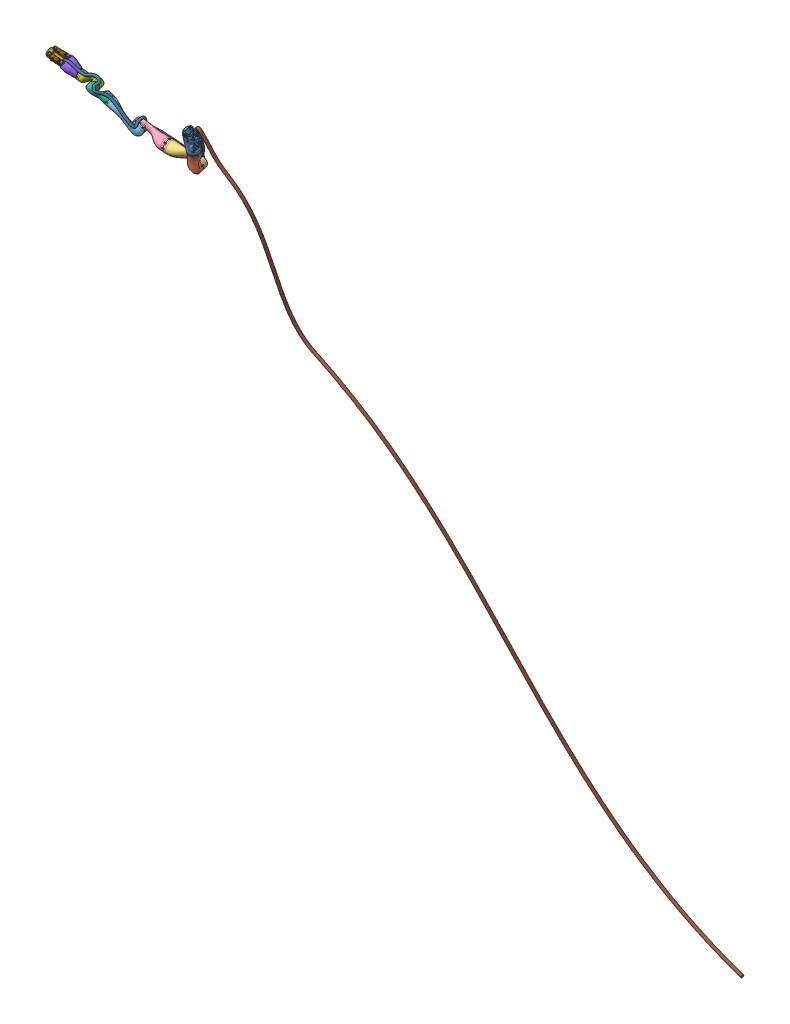
SolidWorks assembly AssemblyWMates_bckp, configuration Default. Lengths in mm.
Overall size (4116.45 4988.8 1804.64).
14 component instances, 12 part files, 30 mates.
Components (placement in the parent):
- Link_1-1: Link_1 [Default] at (138.4866 417.4377 297.5521) x (0.03698 0.287291 -0.957129) z (-0.087201 -0.953203 -0.289482) size (86.63 89.66 156.6)
- Link_2-1: Link_2 [Default] at (138.5302 417.9143 297.6968) x (0.023153 -0.292449 0.956001) z (-0.087201 -0.953203 -0.289482) size (82.77 82.53 159.85)
- Link_3-1: Link_3 [Default] at (387.9844 125.6422 202.7698) x (0.023153 -0.292449 0.956001) z (-0.992619 0.107145 0.056816) size (85.03 82.68 246.21)
- Link_4-1: Link_4 [Default] at (388.4749 125.5421 202.7265) x (0.019798 -0.319039 0.947535) z (-0.992619 0.107145 0.056816) size (85.03 82.68 246.21)
- Link_5-1: Link_5 [Default] at (239.1018 -208.1509 92.9641) x (0.019798 -0.319039 0.947535) z (-0.774729 0.594165 0.216245) size (63.11 82.51 248.26)
- Link_6-1: Link_6 [Default] at (239.5892 -214.9998 111.2165) x (0.009536 0.352942 -0.935597) z (-0.774729 0.594165 0.216245) size (79.26 63.11 135.28)
- Link_7-1: Link_7 [Default] at (435.3893 151.7526 252.0992) x (0.009536 0.352942 -0.935597) z (-0.971222 0.225948 0.075337) size (79.26 63.11 135.28)
- Palm-1: Palm [Default] at (433.6485 146.2609 239.4909) x (0.237886 0.904603 0.353699) z (-0.971222 0.225948 0.075337) size (117.9 99.6 122.71)
- Finger-1: Finger [Default] at (-29.239 -467.0767 -123.4465) x (0.80391 0.582407 0.120544) z (-0.580797 0.725108 0.369991) size (73.19 31.73 75.64)
- Finger-2: Finger [Default] at (319.2901 1059.8577 281.9942) x (0.507306 -0.86175 -0.005255) z (-0.861107 -0.507147 0.036001) size (73.19 31.73 75.64)
- Finger-3: Finger [Default] at (343.0635 944.2648 607.3154) x (0.468613 -0.837857 -0.279995) z (-0.881956 -0.425583 -0.202567) size (73.19 31.73 75.64)
- Part4^AssemblyWMates_bckp-1: Part4^AssemblyWMates_bckp [Default] at (138.4866 417.4377 297.5521) x (-0.03698 -0.287291 0.957129) z (0.087201 0.953203 0.289482) size (166.68 918.69 328.06) (virtual)
- Part5^AssemblyWMates_bckp-1: Part5^AssemblyWMates_bckp [Default] at (134.4689 373.5198 284.2145) x (-0.03698 -0.287291 0.957129) z (0.087201 0.953203 0.289482) size (401.21 3230.32 4793.68) (virtual)
- aruco_marker_holderHose-1: aruco_marker_holderHose [Default] at (-711.4651 422.1788 332.2532) x (0.237886 0.904603 0.353699) z (-0.011767 -0.361442 0.93232) size (60 115.16 60)
Mates (geometry in assembly coordinates):
- Concentric1: concentric anti-aligned: cylinder of Link_2-1 through (124.8397 268.2614 252.2482) axis (0.087201 0.953203 0.289482) radius 37.25; cylinder of Link_1-1 through (124.8397 268.2614 252.2482) axis (-0.087201 -0.953203 -0.289482) radius 37.25
- Coincident2: coincident anti-aligned: plane of Link_2-1 through (86.5196 275.7995 238.97) normal (0.087201 0.953203 0.289482); plane of Link_1-1 through (139.1451 255.8263 288.8854) normal (-0.087201 -0.953203 -0.289482)
- Concentric5: concentric anti-aligned: cylinder of Link_2-1 through (114.4717 155.7455 216.5106) axis (-0.023153 0.292449 -0.956001) radius 37.25; cylinder of Link_3-1 through (114.4717 155.7455 216.5106) axis (0.023153 -0.292449 0.956001) radius 37.25
- Coincident4: coincident anti-aligned: plane of Link_2-1 through (75.1406 143.6201 213.7539) normal (-0.023153 0.292449 -0.956001); plane of Link_3-1 through (134.6777 190.2686 226.5822) normal (0.023153 -0.292449 0.956001)
- Concentric7: concentric anti-aligned: cylinder of Link_3-1 through (-88.7612 177.6103 228.3828) axis (-0.992619 0.107145 0.056816) radius 37.25; cylinder of Link_4-1 through (-88.7612 177.6103 228.3828) axis (0.992619 -0.107145 -0.056816) radius 37.25
- Coincident7: coincident anti-aligned: plane of Link_3-1 through (-83.8589 209.2082 254.4423) normal (-0.992619 0.107145 0.056816); plane of Link_4-1 through (-93.0086 136.6872 231.3523) normal (0.992619 -0.107145 -0.056816)
- Concentric9: concentric anti-aligned: cylinder of Link_4-1 through (-292.0048 199.628 239.779) axis (0.019798 -0.319039 0.947535) radius 37.25; cylinder of Link_5-1 through (-292.0048 199.628 239.779) axis (-0.019798 0.319039 -0.947535) radius 37.25
- Coincident6: coincident anti-aligned: plane of Link_4-1 through (-312.2339 165.4325 228.6879) normal (0.019798 -0.319039 0.947535); plane of Link_5-1 through (-303.8601 162.1096 227.3941) normal (-0.019798 0.319039 -0.947535)
- Concentric11: concentric anti-aligned: cylinder of Link_5-1 through (-452.1511 319.031 295.2016) axis (-0.774729 0.594165 0.216245) radius 29; cylinder of Link_6-1 through (-452.1511 319.031 295.2016) axis (0.774729 -0.594165 -0.216245) radius 29
- Coincident8: coincident anti-aligned: plane of Link_5-1 through (-432.2436 342.2895 302.6169) normal (-0.774729 0.594165 0.216245); plane of Link_6-1 through (-472.066 296.2637 286.4099) normal (0.774729 -0.594165 -0.216245)
- Concentric18: concentric anti-aligned: cylinder of Link_6-1 through (-532.3379 380.4389 317.8169) axis (0.009536 0.352942 -0.935597) radius 29; cylinder of Link_7-1 through (-532.3379 380.4389 317.8169) axis (-0.009536 -0.352942 0.935597) radius 29
- Coincident9: coincident anti-aligned: plane of Link_6-1 through (-552.2529 357.6716 309.0252) normal (0.009536 0.352942 -0.935597); plane of Link_7-1 through (-539.8345 351.8384 306.9513) normal (-0.009536 -0.352942 0.935597)
- Concentric21: concentric anti-aligned: cylinder of Link_7-1 through (-632.8618 403.7363 325.8482) axis (-0.971222 0.225948 0.075337) radius 29; cylinder of Palm-1 through (-632.8618 403.7363 325.8482) axis (0.971222 -0.225948 -0.075337) radius 29
- Coincident10: coincident anti-aligned: plane of Link_7-1 through (-640.3583 375.1358 314.9826) normal (-0.971222 0.225948 0.075337); plane of Palm-1 through (-632.4911 415.1217 296.4801) normal (0.971222 -0.225948 -0.075337)
- Concentric23: concentric aligned: cylinder of Palm-1 through (-750.761 390.7291 342.046) axis (-0.044366 0.533346 -0.844733) radius 1.5; cylinder of Finger-1 through (-752.2779 408.965 313.1634) axis (-0.044366 0.533346 -0.844733) radius 2.5
- Coincident13: coincident anti-aligned: plane of Palm-1 through (-755.2752 408.4531 322.203) normal (-0.044366 0.533346 -0.844733); circle of Finger-1
- Concentric24: concentric aligned: cylinder of Palm-1 through (-738.5394 465.2212 304.6255) axis (0.034765 -0.186428 0.981853) radius 1.5; cylinder of Finger-2 through (-737.3508 458.847 338.1964) axis (0.034765 -0.186428 0.981853) radius 2.5
- Coincident14: coincident anti-aligned: plane of Palm-1 through (-742.6181 457.9619 330.2951) normal (0.034765 -0.186428 0.981853); circle of Finger-2
- Concentric25: concentric aligned: cylinder of Palm-1 through (-737.3339 455.5425 348.472) axis (-0.056567 -0.522567 0.85072) radius 1.5; cylinder of Finger-3 through (-739.268 437.6752 377.5592) axis (-0.056567 -0.522567 0.85072) radius 2.5
- Coincident15: coincident anti-aligned: plane of Palm-1 through (-742.9618 447.7103 356.7051) normal (0.056567 0.522567 -0.85072); circle of Finger-3
- InPlace1: in place: plane of Link_1-1 through (138.4866 417.4377 297.5521) normal (0.087201 0.953203 0.289482); plane of ? through (43.2615 472.8984 143.6161) normal (0.087201 0.953203 0.289482); moOrthogonalPlaneRef_w of Link_1-1 through (138.4866 417.4377 297.5521) normal (0.087201 0.953203 0.289482); plane of ? through (43.2615 472.8984 143.6161) normal (0 0.290588 -0.956848); plane of Link_1-1 through (138.4866 417.4377 297.5521) normal (0.087201 0.953203 0.289482); plane of ? through (43.2615 472.8984 143.6161) normal (0.996191 -0.083438 -0.025339); plane of Link_1-1 through (138.4866 417.4377 297.5521) normal (0.087201 0.953203 0.289482); unknown of Part4^AssemblyWMates_bckp-1
- Coincident17: coincident aligned: plane of Link_1-1; plane of Part4^AssemblyWMates_bckp-1
- Coincident18: coincident aligned: moOrthogonalPlaneRef_w of Link_1-1 through (138.4866 417.4377 297.5521) normal (0.995504 -0.094167 0.010198); plane of Part4^AssemblyWMates_bckp-1 through (138.4866 417.4377 297.5521) normal (0.995504 -0.094167 0.010198)
- Coincident19: coincident anti-aligned: moOrthogonalPlaneRef_w of Link_1-1 through (138.4866 417.4377 297.5521) normal (0.03698 0.287291 -0.957129); plane of Part4^AssemblyWMates_bckp-1 through (138.4866 417.4377 297.5521) normal (-0.03698 -0.287291 0.957129)
- InPlace2: in place: plane of Part4^AssemblyWMates_bckp-1 through (136.0236 385.366 244.739) normal (0.087201 0.953203 0.289482); plane of ? through (39.2438 428.9805 130.2786) normal (0.087201 0.953203 0.289482); plane of Part4^AssemblyWMates_bckp-1 through (136.0236 385.366 244.739) normal (0.087201 0.953203 0.289482); plane of ? through (39.2438 428.9805 130.2786) normal (0 0.290588 -0.956848); plane of Part4^AssemblyWMates_bckp-1 through (136.0236 385.366 244.739) normal (0.087201 0.953203 0.289482); plane of ? through (39.2438 428.9805 130.2786) normal (0.996191 -0.083438 -0.025339); plane of Part4^AssemblyWMates_bckp-1 through (136.0236 385.366 244.739) normal (0.087201 0.953203 0.289482); unknown of Part5^AssemblyWMates_bckp-1
- Coincident20: coincident aligned: plane of Part4^AssemblyWMates_bckp-1; plane of Part5^AssemblyWMates_bckp-1
- Coincident21: coincident aligned: moOrthogonalPlaneRef_w of Part4^AssemblyWMates_bckp-1 through (134.4689 373.5198 284.2145) normal (0.995504 -0.094167 0.010198); plane of Part5^AssemblyWMates_bckp-1 through (134.4689 373.5198 284.2145) normal (0.995504 -0.094167 0.010198)
- Coincident22: coincident anti-aligned: moOrthogonalPlaneRef_w of Part4^AssemblyWMates_bckp-1 through (134.4689 373.5198 284.2145) normal (0.03698 0.287291 -0.957129); plane of Part5^AssemblyWMates_bckp-1 through (134.4689 373.5198 284.2145) normal (-0.03698 -0.287291 0.957129)
- Coincident23: coincident anti-aligned: plane of Palm-1 through (-732.6847 425.0395 332.8471) normal (-0.971222 0.225948 0.075337); plane of aruco_marker_holderHose-1 through (-732.6279 425.1823 333.1505) normal (0.971222 -0.225948 -0.075337)
- Distance1: distance = 10 mm aligned: plane of Palm-1 through (433.6485 146.2609 239.4909) normal (0.237886 0.904603 0.353699); plane of aruco_marker_holderHose-1 through (-711.4651 422.1788 332.2532) normal (0.237886 0.904603 0.353699)
